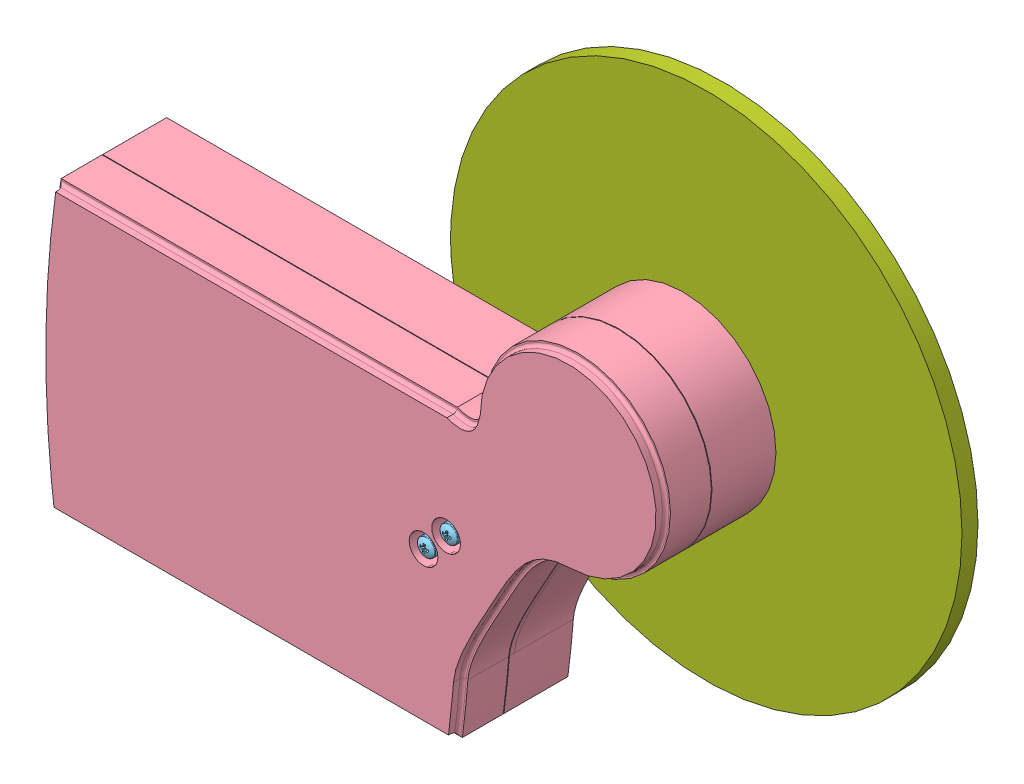
SolidWorks assembly design_assembly, configuration Default. Lengths in mm.
Overall size (257.1 176.37 50.72).
9 component instances, 7 part files, 8 mates.
Components (placement in the parent):
- weight sensor FHDA.step-1: weight sensor FHDA.step [Default] at (88.6115 27.8253 -16.35) x (-0.707107 -0.707107 0) z (-0.707107 0.707107 0) size (82 15.5 15)
- 18650 battery single enclosure.step-1: 18650 battery single enclosure.step [Default] at (-28.8424 2.9903 0) x (0 -1 0) z (1 0 0) size (75.9 20 21.01)
- fabricated_PCB_v1.step-4: fabricated_PCB_v1.step [Default] at (-16.3803 -41.2954 -23.9885) x (1 0 0) z (0 0 1) size (61.21 84.93 14.61)
- enclosure-1: enclosure [Default] at origin size (206.1 125.37 38.52)
- pan head cross recess screw_iso-2: pan head cross recess screw_iso [ISO 7045 - M3 x 30 - Z - 25C] at (65.9841 5.1978 4.5) x (0 0 -1) z (0.087784 0.99614 0) size (32.35 5.6 5.6)
- pan head cross recess screw_iso-4: pan head cross recess screw_iso [ISO 7045 - M3 x 30 - Z - 25C] at (73.0552 12.2689 4.5) x (0 0 -1) z (0.079445 0.996839 0) size (32.35 5.6 5.6)
- hex nut style 1 gradeab_iso-1: hex nut style 1 gradeab_iso [ISO - 4032 - M5 - W - N] at (73.0552 12.2689 -22.7) size (8 9.24 4.7)
- hex nut style 1 gradeab_iso-2: hex nut style 1 gradeab_iso [ISO - 4032 - M5 - W - N] at (65.9841 5.1978 -22.7) size (8 9.24 4.7)
- tray-1: tray [Default] at origin size (160 160 21)
Mates (geometry in assembly coordinates):
- Lock1: lock: unknown of weight sensor FHDA.step-1; unknown of enclosure-1
- Lock2: lock: unknown of 18650 battery single enclosure.step-1; unknown of enclosure-1
- Lock3: lock: unknown of fabricated_PCB_v1.step-4; unknown of enclosure-1
- Concentric2: concentric aligned: circle of enclosure-1; circle of pan head cross recess screw_iso-4
- Concentric7: concentric aligned: cylinder of pan head cross recess screw_iso-4 through (73.0552 12.2689 29.9) axis (0 0 1) radius 1.5; cylinder of hex nut style 1 gradeab_iso-1 through (73.0552 12.2689 -47.7375) axis (0 0 1) radius 2.5
- Concentric8: concentric aligned: cylinder of pan head cross recess screw_iso-2 through (65.9841 5.1978 29.9) axis (0 0 1) radius 1.5; cylinder of hex nut style 1 gradeab_iso-2 through (65.9841 5.1978 -47.7375) axis (0 0 1) radius 2.5
- Coincident7: coincident anti-aligned: plane of weight sensor FHDA.step-1 through (110.6379 58.8319 -22.7) normal (0 0 -1); plane of hex nut style 1 gradeab_iso-1 through (65.0552 12.2689 -22.7) normal (0 0 1)
- Coincident8: coincident anti-aligned: plane of weight sensor FHDA.step-1 through (110.6379 58.8319 -22.7) normal (0 0 -1); plane of hex nut style 1 gradeab_iso-2 through (57.9841 5.1978 -22.7) normal (0 0 1)
